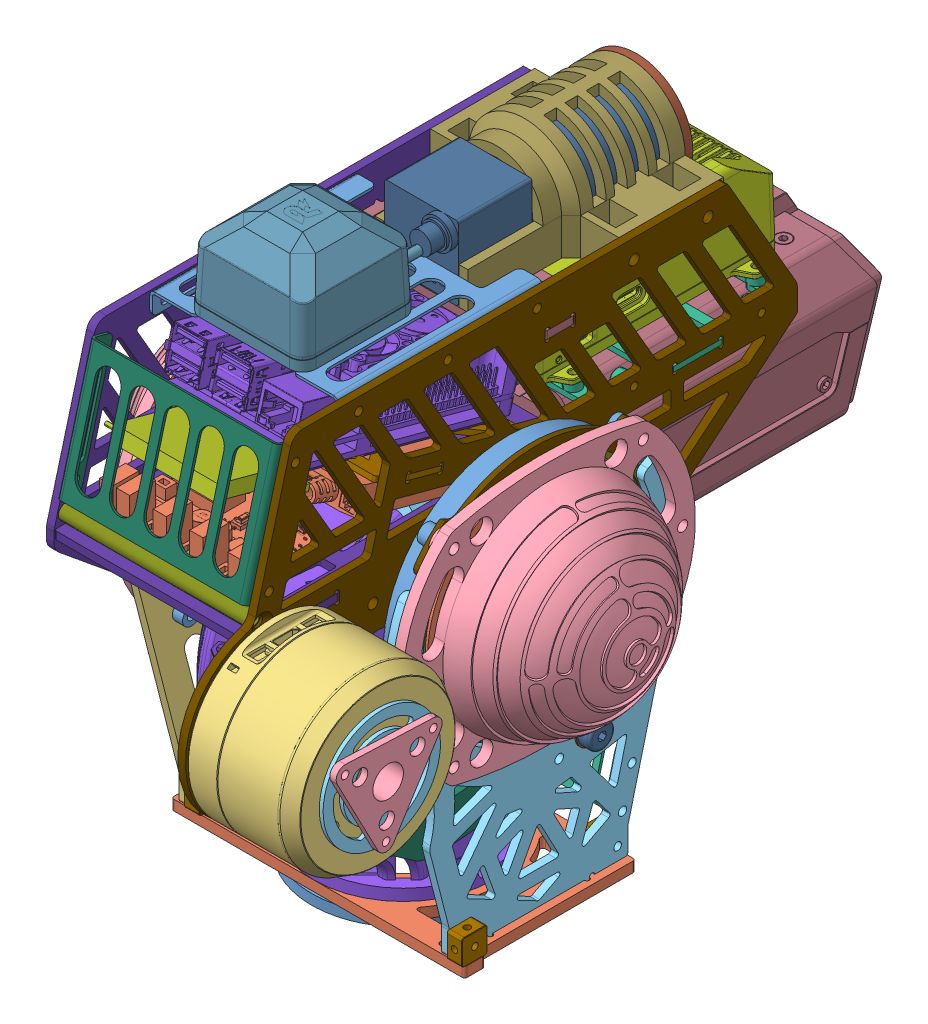
SolidWorks assembly 云台-耳机云台2.0, configuration 默认. Lengths in mm.
Overall size (183.97 237.5 278.23).
99 component instances, 56 part files, 14 mates.
Components (placement in the parent):
- yaw轴底部垫板-1: yaw轴底部垫板 [默认] at origin size (72 4 72)
- yaw轴框架-1: yaw轴框架 [默认] at (0 4 0) size (183.97 157 120.25)
  - yaw轴框架基板-1: yaw轴框架基板 [默认] at origin size (115 4 70)
  - yaw轴框架板-左-3: yaw轴框架板-左 [默认] at (-53 109 0) x (0 0 -1) z (0 -1 0) size (115 3 134.47)
  - 摩擦轮保护打印-1: 摩擦轮保护打印 [默认] at (-50 109 0) size (39.98 96 115)
  - 摩擦轮保护打印-2: 摩擦轮保护打印 [默认] at (50 109 0) x (-1 0 0) z (0 0 -1) size (39.98 96 115)
  - yaw轴框架板-右-5: yaw轴框架板-右 [默认] at (50 109 0) x (0 0 -1) z (0 -1 0) size (115 3 134.47)
  - yaw轴框架前部钣金-1: yaw轴框架前部钣金 [默认] at (0 26.1472 -39.1472) x (1 0 0) z (0 -0.968661 0.248388) size (100 9 25)
  - 连杆安装垫板-1: 连杆安装垫板 [默认] at (50 54.4978 -19.8372) x (0 -0.34202 0.939693) z (-1 0 0) size (33 14 3)
  - 云台弹链打印-1: 云台弹链打印 [默认] at (0 8.5 0) x (-1 0 0) z (0 0 -1) size (70 127.19 97.75)
  - 六面螺母10×10×6-M3-1: 六面螺母10×10×6-M3 [默认] at (-47 9 -31) x (0 -1 0) z (0 0 1) size (10 6 10)
  - 六面螺母10×10×6-M3-2: 六面螺母10×10×6-M3 [默认] at (-47 9 31) x (0 -1 0) z (0 0 1) size (10 6 10)
  - 六面螺母10×10×6-M3-3: 六面螺母10×10×6-M3 [默认] at (47 9 -31) x (0 -1 0) z (0 0 -1) size (10 6 10)
  - 六面螺母10×10×6-M3-4: 六面螺母10×10×6-M3 [默认] at (56 9 31) x (0 -1 0) z (0 0 1) size (10 6 10)
- pitch轴-1: pitch轴 [默认] at (0 113 0) x (-1 0 0) z (0 0 -1) size (166 173.82 278.23)
  - pitch轴大发射-1: pitch轴大发射 [默认] at origin size (160 95.03 252.73)
    - 摩擦轮-1: 摩擦轮 [默认] at origin size (160 20 60)
    - 发射机构底板-1: 发射机构底板 [默认] at (0 -28 0) x (-1 0 0) z (0 0 -1) size (123 3 59.75)
    - M3508电机无减速箱-1: M3508电机无减速箱 [默认] at (50 61 0) x (-0.707107 0 0.707107) z (-0.707107 0 -0.707107) size (42 43.4 42)
    - RM2019裁判系统测速模块SM11-1: RM2019裁判系统测速模块SM11 [默认] at (21.5261 -69.6659 -28.7637) size (74 74 119.73)
    - 测速模块卡板-1: 测速模块卡板 [默认] at (21.5261 -69.6659 -28.7637) size (2 31.6 11.8)
    - 摩擦轴承连接法兰-1: 摩擦轴承连接法兰 [默认] at (50 -10 0) x (-1 0 0) z (0 0 1) size (27.52 19.2 26)
    - 法兰轴承F6700zz-10x15x4-16.5x0.8-1: 法兰轴承F6700zz-10x15x4-16.5x0.8 [默认] at (50 -28.2 0) x (0 1 0) z (-0.223049 0 -0.974807) size (4 16.5 16.5)
    - 摩擦轮安装板-1: 摩擦轮安装板 [默认] at (0 25 0) x (-1 0 0) z (0 0 -1) size (142 3 133)
    - 法兰轴承F6700zz-10x15x4-16.5x0.8-2: 法兰轴承F6700zz-10x15x4-16.5x0.8 [默认] at (-50 -28.2 0) x (0 1 0) z (-0.223049 0 0.974807) size (4 16.5 16.5)
    - 摩擦轴承连接法兰-2: 摩擦轴承连接法兰 [默认] at (-50 -10 0) x (-1 0 0) z (0 0 1) size (27.52 19.2 26)
    - M3508电机无减速箱-3: M3508电机无减速箱 [默认] at (-50 61 0) x (-0.707107 0 -0.707107) z (0.707107 0 -0.707107) size (42 43.4 42)
    - hexagon socket head cap screws gb-3: hexagon socket head cap screws gb [GB_FASTENER_SCREWS_HSHCS M3X6-C] at (43.5 -10.1 0) x (0 1 0) z (0.546944 0 -0.837169) size (9 5.5 5.5)
    - hexagon socket head cap screws gb-4: hexagon socket head cap screws gb [GB_FASTENER_SCREWS_HSHCS M3X6-C] at (56.5 -10.1 0) x (0 1 0) z (0.546944 0 -0.837169) size (9 5.5 5.5)
    - hexagon socket head cap screws gb-5: hexagon socket head cap screws gb [GB_FASTENER_SCREWS_HSHCS M3X6-C] at (38.7417 -15 6.5) x (0 1 0) z (0.524684 0 -0.851297) size (9 5.5 5.5)
    - hexagon socket head cap screws gb-6: hexagon socket head cap screws gb [GB_FASTENER_SCREWS_HSHCS M3X6-C] at (61.2583 -15 6.5) x (0 1 0) z (0.546944 0 -0.837169) size (9 5.5 5.5)
    - hexagon socket head cap screws gb-7: hexagon socket head cap screws gb [GB_FASTENER_SCREWS_HSHCS M3X6-C] at (50 -15 -13) x (0 1 0) z (0.546944 0 -0.837169) size (9 5.5 5.5)
    - 镜向测速模块固定打印件-2: 镜向测速模块固定打印件 [默认] at (-21.5261 -69.6659 -28.7637) x (-1 0 0) z (0 0 -1) size (2 31.6 11.8)
    - hexagon socket head cap screws gb-8: hexagon socket head cap screws gb [GB_FASTENER_SCREWS_HSHCS M3X6-C] at (-61.2583 -15 6.5) x (0 1 0) z (0.546944 0 0.837169) size (9 5.5 5.5)
    - hexagon socket head cap screws gb-9: hexagon socket head cap screws gb [GB_FASTENER_SCREWS_HSHCS M3X6-C] at (-38.7417 -15 6.5) x (0 1 0) z (0.524684 0 0.851297) size (9 5.5 5.5)
    - hexagon socket head cap screws gb-10: hexagon socket head cap screws gb [GB_FASTENER_SCREWS_HSHCS M3X6-C] at (-50 -15 -13) x (0 1 0) z (0.546944 0 0.837169) size (9 5.5 5.5)
    - hexagon socket head cap screws gb-11: hexagon socket head cap screws gb [GB_FASTENER_SCREWS_HSHCS M3X6-C] at (-43.5 -10.1 0) x (0 1 0) z (0.546944 0 0.837169) size (9 5.5 5.5)
    - hexagon socket head cap screws gb-12: hexagon socket head cap screws gb [GB_FASTENER_SCREWS_HSHCS M3X6-C] at (-56.5 -10.1 0) x (0 1 0) z (0.546944 0 0.837169) size (9 5.5 5.5)
    - Hero_Master-1: Hero_Master [默认] at (28 31.4115 -92) x (-1 0 0.000001) z (0 1 0) size (56 41.25 17)
    - spur gear_gb-1: spur gear_gb [GB - Spur gear 0.6M 16T 20PA 6.5FW ---S16A75H50L5.0N] at (50 33.5 0) x (0 -1 0) z (0 0 1) size (6.5 10.64 10.64)
    - spur gear_gb-2: spur gear_gb [GB - Spur gear 0.6M 16T 20PA 6.5FW ---S16A75H50L5.0N] at (-50 33.5 0) x (0 -1 0) z (0 0 -1) size (6.5 10.64 10.64)
    - RoboMaster 红点激光器-1: RoboMaster 红点激光器 [默认] at (20.4617 -46.413 101.4662) x (-1 0 0) z (0 0 1) size (25 20.86 51.36)
    - 炮管-1: 炮管 [默认] at (0 0 33) size (50 55.5 52)
  - pitch轴顶部设备-1: pitch轴顶部设备 [默认] at (0 37 75.5) x (-1 0 0) z (0 0 -1) size (80.14 158 249.05)
    - 图传安装架-1: 图传安装架 [默认] at origin size (80 6 78)
    - RM2019图传模块VT02-1: RM2019图传模块VT02 [默认] at (0 5 0.35) size (60 36.09 100.47)
    - Raspberry Pi 4 Model B-1: Raspberry Pi 4 Model B [默认] at (0 22.2544 100.0052) x (0 0.258819 0.965926) z (-1 0 0) size (93.45 25.9 58.4)
    - 树莓派安装板-1: 树莓派安装板 [默认] at (0 9.8234 92.9833) x (1 0 0) z (0 0.258819 0.965926) size (80 2 64)
    - 相机MER-139-210U3C;HN-0612-2M-C1÷2X-1: 相机MER-139-210U3C;HN-0612-2M-C1÷2X [默认] at (0 53.5 39.5) x (0 1 0) z (1 0 0) size (32.45 89.5 29.5)
    - 相机顶部保护PC板-1: 相机顶部保护PC板 [默认] at (0 53.5 -13) x (-1 0 0) z (0 0 -1) size (44 38.5 3)
    - 相机顶部保护壳-1: 相机顶部保护壳 [默认] at (0 53.5 39) x (1 0 0) z (0 0 -1) size (74 36.5 81.5)
    - 相机顶部安装板-1: 相机顶部安装板 [默认] at (0 36 39.5) size (80 3 29)
    - hexagon socket head cap screws gb-1: hexagon socket head cap screws gb [GB_FASTENER_SCREWS_HSHCS M3X6-C] at (-10 33 41.8) x (0 1 0) z (0 0 -1) size (9 5.5 5.5)
    - hexagon socket head cap screws gb-3: hexagon socket head cap screws gb [GB_FASTENER_SCREWS_HSHCS M3X6-C] at (10 33 41.8) x (0 1 0) z (0 0 -1) size (9 5.5 5.5)
    - RM2019裁判系统定位模块UW01-1: RM2019裁判系统定位模块UW01 [默认] at (0 54 115) x (-1 0 0) z (0 0 -1) size (45.56 33.5 81.86)
    - 后端钣金支撑-1: 后端钣金支撑 [默认] at (0 25.3462 167.3322) x (1 0 0) z (0 0.965926 -0.258819) size (74 9 50)
    - 铝柱M4×74-定制-1: 铝柱M4×74-定制 [默认] at (37 -5 62.5) x (0 0 1) z (-1 0 0) size (6 6 74)
    - 铝柱M4×74-定制-2: 铝柱M4×74-定制 [默认] at (37 -5 170.8047) x (0 0.986463 -0.163981) z (-1 0 0) size (6 6 74)
    - pitch轴外框竖板-1: pitch轴外框竖板 [默认] at (-37 -37 75.5) x (-1 0 0) z (0 0 -1) size (3 124 214.5)
    - pitch轴外框竖板-电机-1: pitch轴外框竖板-电机 [默认] at (40 -37 75.5) x (-1 0 0) z (0 0 -1) size (3.14 124 240)
    - 顶部钣金支撑-1: 顶部钣金支撑 [默认] at (0 53 98) x (-1 0 0) z (0 0 1) size (74 9 80)
  - C620无刷电机调速器-1: C620无刷电机调速器 [默认] at (24.1 44.998 -31.5346) x (0 -0.258819 0.965926) z (-1 0 0) size (53.7 11.5 26.13)
  - GM6020 直流无刷电机-1: GM6020 直流无刷电机 [默认] at (-40 0 -92) x (0 0 -1) z (0 1 0) size (66.7 45 66.7)
  - C620无刷电机调速器-2: C620无刷电机调速器 [默认] at (-23.7747 44.998 -31.5346) x (0 -0.258819 0.965926) z (-1 0 0) size (53.7 11.5 26.13)
  - 6020驱动轴-pitch-1: 6020驱动轴-pitch [默认] at (-86 0 -92) x (0 0.844933 0.534871) z (0 0.534871 -0.844933) size (41.64 53 37)
  - 6020转子垫板-1: 6020转子垫板 [默认] at (-82 0 -92) x (0 0.844933 0.534871) z (-1 0 0) size (46 46 1.5)
  - hexagon socket button head screws gb-1: hexagon socket button head screws gb [GB_SOCKET_TYPE7 M5X10-C] at (-34.25 -29 -92) x (-1 0 0) z (0 0.924225 0.381849) size (12.75 9.5 9.5)
  - DR16接收机-1: DR16接收机 [默认] at (49.7211 -0.2116 264.9782) x (0.063491 0.963645 0.259534) z (-0.997779 0.066551 -0.00301) size (8.23 30.82 54.76)
  - 六面螺母10×10×10-M3-1: 六面螺母10×10×10-M3 [默认] at (32 -20 19.25) size (10 10 10)
  - 六面螺母10×10×10-M3-3: 六面螺母10×10×10-M3 [默认] at (32 -20 -19.25) size (10 10 10)
  - 六面螺母10×10×10-M3-4: 六面螺母10×10×10-M3 [默认] at (-32 -20 -19.25) x (-1 0 0) z (0 0 -1) size (10 10 10)
  - 六面螺母10×10×10-M3-5: 六面螺母10×10×10-M3 [默认] at (-32 -20 19.25) x (-1 0 0) z (0 0 -1) size (10 10 10)
- 连杆-1: 连杆 [默认] at (33 113 92) x (0 0.34202 -0.939693) z (1 0 0) size (112.09 123.32 35.37) (flexible)
  - 连杆摇杆-1: 连杆摇杆 [默认] x (-1 0 0) z (0 0 -1) size (19 76 5)
  - 轴肩螺栓 O6xM5x16-1: 轴肩螺栓 O6xM5x16 [默认] at (0 -58 -10.2732) x (0 0 1) z (0.240236 0.970714 0) size (30.5 10 10)
  - 法兰轴承MF106ZZ-6×10×3-11.2×0.6-1: 法兰轴承MF106ZZ-6×10×3-11.2×0.6 [默认] at (0 -58 -5.6) x (-0.983645 -0.180119 0) z (-0.180119 0.983645 0) size (11.2 3 11.2)
  - 推力球轴承F6-12M 6x12x4.5-1: 推力球轴承F6-12M 6x12x4.5 [默认] at (0 -58 0) x (0.638605 -0.769535 0) z (0 0 1) size (12 12 4.5)
  - 法兰轴承MF106ZZ-6×10×3-11.2×0.6-2: 法兰轴承MF106ZZ-6×10×3-11.2×0.6 [默认] at (0 -58 10.1) x (0.628312 -0.777961 0) z (0.777961 0.628312 0) size (11.2 3 11.2)
  - prevailing torque type 2 gb-1: prevailing torque type 2 gb [GB_HEXAGON_LOCK_TYPE10 M5-N] at (0 -58 15.12) x (0.98026 -0.197711 0) z (0 0 1) size (9.24 8 7.2)
  - 推力球轴承F6-12M 6x12x4.5-3: 推力球轴承F6-12M 6x12x4.5 [默认] at (86.4517 -89.4659 14) x (-0.218092 0.975928 0) z (0 0 -1) size (12 12 4.5)
  - 法兰轴承MF106ZZ-6×10×3-11.2×0.6-5: 法兰轴承MF106ZZ-6×10×3-11.2×0.6 [默认] at (86.4517 -89.4659 3.9) x (0.335901 0.941897 0) z (0.941897 -0.335901 0) size (11.2 3 11.2)
  - M6尼龙垫圈-5: M6尼龙垫圈 [默认] at (0 -58 10.1) x (-0.999887 -0.015047 0) z (-0.015047 0.999887 0) size (12 1.5 12)
  - 联杆-长杆-2: 联杆-长杆 [默认] at (0 -58 4.5) x (0.939693 -0.34202 0) z (-0.34202 -0.939693 0) size (108 5 31.01)
  - 法兰轴承MF106ZZ-6×10×3-11.2×0.6-6: 法兰轴承MF106ZZ-6×10×3-11.2×0.6 [默认] at (86.4517 -89.4659 20.6) x (-0.817308 0.576202 0) z (-0.576202 -0.817308 0) size (11.2 3 11.2)
  - 轴肩螺栓 O6xM5x16-4: 轴肩螺栓 O6xM5x16 [默认] at (86.4517 -89.4659 25.1) x (0 0 -1) z (0.997178 -0.075079 0) size (30.5 10 10)
- pitch轴系-1: pitch轴系 [默认] at (-42 113 0) x (0 -1 0) z (0 0 -1) size (100.05 18 112) (flexible)
  - 薄壁轴承K08008-80×96×8-1: 薄壁轴承K08008-80×96×8 [默认] x (0.999901 0 -0.014042) z (0.014042 0 0.999901) size (96 8 96)
  - pitch轴轴承内圈垫板-1: pitch轴轴承内圈垫板 [默认] at (0 -2 0) x (0 1 0) z (0 0 1) size (2 85.9 85.9)
  - pitch轴轴承外圈垫板-1: pitch轴轴承外圈垫板 [默认] at (0 8 0) x (0 0 -1) z (1 0 0) size (92.03 2 26.47)
  - pitch轴轴承外圈-1: pitch轴轴承外圈 [默认] at (0 8 0) x (0 0 1) z (1 0 0) size (112 9 98)
  - pitch轴轴承内圈-1: pitch轴轴承内圈 [默认] at (0 9 0) x (0 0 -1) z (-1 0 0) size (83 9 83)
  - hexagon socket head cap screws gb-5: hexagon socket head cap screws gb [GB_FASTENER_SCREWS_HSHCS M4X8-C] at (-32 4 13) x (0 -1 0) z (-0.819152 0 -0.573576) size (12 7 7)
- pitch轴系-2: pitch轴系 [默认] at (42 113 0) x (0 -1 0) z (0 0 1) size (100.05 18 112) (flexible)
  - 薄壁轴承K08008-80×96×8-1: 薄壁轴承K08008-80×96×8 [默认] x (0.999901 0 -0.014042) z (0.014042 0 0.999901) size (96 8 96)
  - pitch轴轴承内圈垫板-1: pitch轴轴承内圈垫板 [默认] at (0 -2 0) x (0 1 0) z (0 0 1) size (2 85.9 85.9)
  - pitch轴轴承外圈垫板-1: pitch轴轴承外圈垫板 [默认] at (0 8 0) x (0 0 -1) z (1 0 0) size (92.03 2 26.47)
  - pitch轴轴承外圈-1: pitch轴轴承外圈 [默认] at (0 8 0) x (0 0 1) z (1 0 0) size (112 9 98)
  - pitch轴轴承内圈-1: pitch轴轴承内圈 [默认] at (0 9 0) x (0 0 -1) z (-1 0 0) size (83 9 83)
  - hexagon socket head cap screws gb-5: hexagon socket head cap screws gb [GB_FASTENER_SCREWS_HSHCS M4X8-C] at (-32 4 13) x (0 -1 0) z (-0.819152 0 -0.573576) size (12 7 7)
Mates (geometry in assembly coordinates):
- 同心16: concentric: cylinder of yaw轴底部垫板-1 through (0 4 0) axis (0 -1 0) radius 22; cylinder of yaw轴框架-1/yaw轴框架基板-1 through (0 4 0) axis (0 1 0) radius 21.5
- 同心17: concentric: cylinder of yaw轴底部垫板-1 through (0 4 30) axis (0 -1 0) radius 2; cylinder of yaw轴框架-1/yaw轴框架基板-1 through (0 4 30) axis (0 1 0) radius 2
- 重合10: coincident: plane of yaw轴底部垫板-1 through (0 4 0) normal (0 1 0); plane of yaw轴框架-1/yaw轴框架基板-1 through (0 4 0) normal (0 -1 0)
- LimitAngle1: limit planar angle = 0 rad: plane of pitch轴-1/pitch轴大发射-1/发射机构底板-1 through (-50 85 0) normal (0 -1 0); plane of yaw轴框架-1/yaw轴框架基板-1 through (0 8 0) normal (0 1 0)
- 同心84: concentric: cylinder of pitch轴-1/pitch轴顶部设备-1/pitch轴外框竖板-1 through (-40 130.75 -30.7439) axis (1 0 0) radius 2; cylinder of pitch轴系-1/pitch轴轴承内圈垫板-1 through (-42 130.75 -30.7439) axis (1 0 0) radius 2
- 同心85: concentric: cylinder of pitch轴-1/pitch轴顶部设备-1/pitch轴外框竖板-1 through (-40 95.25 -30.7439) axis (1 0 0) radius 2; cylinder of pitch轴系-1/pitch轴轴承内圈垫板-1 through (-42 95.25 -30.7439) axis (1 0 0) radius 2
- 重合64: coincident: plane of pitch轴-1/pitch轴顶部设备-1/pitch轴外框竖板-1 through (-40 198.5 79.4165) normal (-1 0 0); plane of pitch轴系-1/pitch轴轴承内圈垫板-1 through (-40 113 0) normal (1 0 0)
- 同心98: concentric: cylinder of yaw轴框架-1/yaw轴框架板-左-3 through (-50 113 0) axis (-1 0 0) radius 45.5; cylinder of pitch轴系-1/pitch轴轴承内圈-1 through (-51 113 0) axis (-1 0 0) radius 39
- 同心99: concentric: cylinder of pitch轴系-1/pitch轴轴承外圈-1 through (-50 113 -52.5) axis (-1 0 0) radius 1.65; cylinder of yaw轴框架-1/yaw轴框架板-左-3 through (-50 113 -52.5) axis (-1 0 0) radius 2
- 重合88: coincident: plane of pitch轴-1/pitch轴大发射-1/摩擦轮-1 through (0 113 0) normal (-1 0 0); plane of assembly through (0 0 0) normal (1 0 0)
- 同心100: concentric: cylinder of pitch轴-1/6020驱动轴-pitch-1 through (86 113 92) axis (-1 0 0) radius 4; cylinder of 连杆-1/连杆摇杆-1 through (28 113 92) axis (1 0 0) radius 2
- 重合90: coincident: plane of pitch轴系-1/pitch轴轴承外圈-1 through (-50 113 0) normal (0 0 -1); plane of pitch轴系-2/pitch轴轴承外圈-1 through (50 113 0) normal (0 0 1)
- 同心101: concentric: cylinder of yaw轴框架-1/yaw轴框架板-右-5 through (53 58.4978 -19.8372) axis (-1 0 0) radius 5.1; cylinder of 连杆-1/法兰轴承MF106ZZ-6×10×3-11.2×0.6-6 through (50.6 58.4978 -19.8372) axis (1 0 0) radius 5
- 重合93: coincident: plane of yaw轴框架-1/连杆安装垫板-1 through (47 62.7731 -31.5833) normal (-1 0 0); plane of 连杆-1/推力球轴承F6-12M 6x12x4.5-3 through (47 58.4978 -19.8372) normal (1 0 0)
